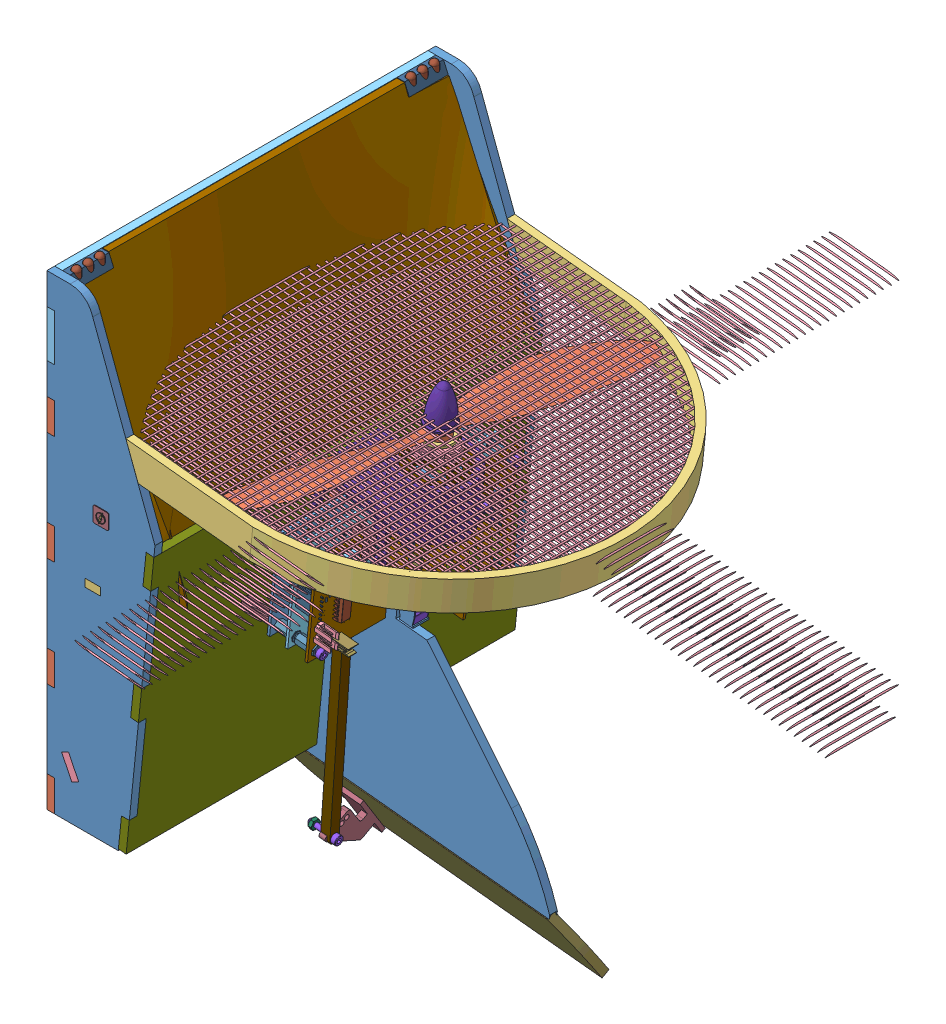
SolidWorks assembly AssTotaleSimu2, configuration Défaut. Lengths in mm. (continued)
Components (placement in the parent): (continued)
- AssStructSimu-1: AssStructSimu [Défaut] at (-125.7658 -1.8483 624.6548) x (1 0 0) z (0 0 -1) size (253.25 324.59 251.6) (continued)
  - AssCarte-1: AssCarte [Défaut] at (38.0121 147.1029 290.772) x (-0.101852 0.9948 0) z (0.9948 0.101852 0) size (66.52 130.57 98.72) (continued)
    - carte_onduleur_v3-1: carte_onduleur_v3 [Défaut] at (-131.8199 12.0892 20.7912) size (66.52 130.57 82.34) (continued)
      - RC2_2-1: RC2_2 [Défaut] at (-22 0.18 -0.803) x (-1 0 0) z (0 0 -1) size (2.34 1.04 0.5) (continued)
        - Open CASCADE STEP translator 6.8 1.12.1-1: Open CASCADE STEP translator 6.8 1.12.1 [Défaut] at origin size (2.34 1.04 0.5) (continued)
          - Pin_2_2-1: Pin_2_2 [Défaut] at origin size (0.51 1.02 0.5)
      - RC3_1-1: RC3_1 [Défaut] at (-20.9336 -14.5 -0.803) x (1 0 0) z (0 0 -1) size (2.34 1.04 0.5)
        - Open CASCADE STEP translator 6.8 1.12.1-1: Open CASCADE STEP translator 6.8 1.12.1 [Défaut] at origin size (2.34 1.04 0.5)
          - Body_1_3-1: Body_1_3 [Défaut] at origin size (2.29 1.04 0.43)
          - Pin_1_2-1: Pin_1_2 [Défaut] at (0.3048 0 0) x (-1 0 0) z (0 0 1) size (0.51 1.02 0.5)
          - Pin_2_2-1: Pin_2_2 [Défaut] at origin size (0.51 1.02 0.5)
      - RC3_2-1: RC3_2 [Défaut] at (-22.3 -14.5 -0.803) x (-1 0 0) z (0 0 -1) size (2.34 1.04 0.5)
        - Open CASCADE STEP translator 6.8 1.12.1-1: Open CASCADE STEP translator 6.8 1.12.1 [Défaut] at origin size (2.34 1.04 0.5)
          - Body_1_3-1: Body_1_3 [Défaut] at origin size (2.29 1.04 0.43)
          - Pin_1_2-1: Pin_1_2 [Défaut] at (0.3048 0 0) x (-1 0 0) z (0 0 1) size (0.51 1.02 0.5)
          - Pin_2_2-1: Pin_2_2 [Défaut] at origin size (0.51 1.02 0.5)
      - U_MES_CUR-1: U_MES_CUR [Défaut] at (-11.5 6.7816 0.803) size (2.54 2.41 0.76)
        - Open CASCADE STEP translator 6.8 1.32.1-1: Open CASCADE STEP translator 6.8 1.32.1 [Défaut] at origin size (2.54 2.41 0.76)
          - Body_1_5-1: Body_1_5 [Défaut] at origin size (2.54 1.27 0.71)
          - Pin_1_3-1: Pin_1_3 [Défaut] at (-2.1082 0.2286 0) x (0 -1 0) z (0 0 1) size (1.14 0.25 0.47)
          - Pin_2_3-1: Pin_2_3 [Défaut] at (-0.2032 2.1336 0) x (0 -1 0) z (0 0 1) size (1.14 0.25 0.47)
      - CARTE_ALIM-1: CARTE_ALIM [Défaut] at (-6.4 -57.2 0.803) size (60 130 18.35)
        - Open CASCADE STEP translator 6.8 1.33.1-1: Open CASCADE STEP translator 6.8 1.33.1 [Défaut] at origin size (60 130 18.35)
          - Body_1_6-1: Body_1_6 [Défaut] at (7 56 -12) size (60 130 18.35)
            - 1_3-1: 1_3 [Défaut] at origin size (60 130 1.61)
            - 13_3-1: 13_3 [Défaut] at (0.4717 -40.93 0.803) x (0 1 0) z (0 0 1) size (5.65 4.9 1.7)
              - =_[0_1_1_4]_3-1: =_[0_1_1_4]_3 [Défaut] at origin size (5.65 4.9 1.7)
                - 2-1: 2 [Défaut] at origin size (3.75 4.9 1.53)
                - 3-1: 3 [Défaut] at origin size (0.95 0.51 1.06)
                - 4-1: 4 [Défaut] at origin size (0.95 0.51 1.06)
                - 5_2-1: 5_2 [Défaut] at origin size (0.95 0.51 1.06)
                - 6-1: 6 [Défaut] at origin size (0.95 0.51 1.06)
                - 7-1: 7 [Défaut] at (10.8 -5.08 0) x (-1 0 0) z (0 0 1) size (0.95 0.51 1.06)
                - 8_2-1: 8_2 [Défaut] at (10.8 -2.54 0) x (-1 0 0) z (0 0 1) size (0.95 0.51 1.06)
                - 9-1: 9 [Défaut] at (10.8 0 0) x (-1 0 0) z (0 0 1) size (0.95 0.51 1.06)
                - 10-1: 10 [Défaut] at (10.8 2.54 0) x (-1 0 0) z (0 0 1) size (0.95 0.51 1.06)
                - 11_2-1: 11_2 [Défaut] at (5.4 -1.27 0) x (-1 0 0) z (0 0 1) size (4.25 2.34 1.06)
            - 18-1: 18 [Défaut] at (-2.5283 -37.23 0.803) x (0 -1 0) z (0 0 1) size (2.34 1.04 0.5)
              - =_[0_1_1_16]-1: =_[0_1_1_16] [Défaut] at origin size (2.34 1.04 0.5)
                - 14_2-1: 14_2 [Défaut] at origin size (2.29 1.04 0.43)
                - 15_2-1: 15_2 [Défaut] at (0.3048 0 0) x (-1 0 0) z (0 0 1) size (0.51 1.02 0.5)
                - 16_2-1: 16_2 [Défaut] at origin size (0.51 1.02 0.5)
            - 21_2-1: 21_2 [Défaut] at (-2.2263 -24.628 -0.803) x (1 0 0) z (0 0 -1) size (8.01 8 14.24)
              - =_[0_1_1_21]-1: =_[0_1_1_21] [Défaut] at origin size (8.01 8 14.24)
                - 19-1: 19 [Défaut] at (1.8 0 0) x (1 0 0) z (0 -1 0) size (8.01 14.24 8)
            - 23_2-1: 23_2 [Défaut] at (1.2381 -31.53 0.803) size (2.34 1.04 0.5)
              - =_[0_1_1_16]-1: =_[0_1_1_16] [Défaut] at origin size (2.34 1.04 0.5)
                - 14_2-1: 14_2 [Défaut] at origin size (2.29 1.04 0.43)
                - 15_2-1: 15_2 [Défaut] at (0.3048 0 0) x (-1 0 0) z (0 0 1) size (0.51 1.02 0.5)
                - 16_2-1: 16_2 [Défaut] at origin size (0.51 1.02 0.5)
            - 28-1: 28 [Défaut] at (5 29.8636 0.803) x (0 -1 0) z (0 0 1) size (3.35 1.3 0.55)
              - =_[0_1_1_25]_2-1: =_[0_1_1_25]_2 [Défaut] at origin size (3.35 1.3 0.55)
                - 24-1: 24 [Défaut] at origin size (3.3 1.3 0.48)
                - 25_2-1: 25_2 [Défaut] at (0.5588 0 0) x (-1 0 0) z (0 0 1) size (0.76 1.27 0.55)
                - 26_2-1: 26_2 [Défaut] at origin size (0.76 1.27 0.55)
            - 30-1: 30 [Défaut] at (6.7 29.8636 0.803) x (0 -1 0) z (0 0 1) size (2.34 1.04 0.5)
              - =_[0_1_1_16]-1: =_[0_1_1_16] [Défaut] at origin size (2.34 1.04 0.5)
                - 14_2-1: 14_2 [Défaut] at origin size (2.29 1.04 0.43)
                - 15_2-1: 15_2 [Défaut] at (0.3048 0 0) x (-1 0 0) z (0 0 1) size (0.51 1.02 0.5)
                - 16_2-1: 16_2 [Défaut] at origin size (0.51 1.02 0.5)
            - 35_2-1: 35_2 [Défaut] at (-2.5 -46.37 0.803) x (0 1 0) z (0 0 1) size (3.4 2.06 0.79)
              - =_[0_1_1_31]-1: =_[0_1_1_31] [Défaut] at origin size (3.4 2.06 0.79)
                - 31_2-1: 31_2 [Défaut] at origin size (3.3 2.06 0.69)
                - 32_3-1: 32_3 [Défaut] at (0.5588 0 0) x (-1 0 0) z (0 0 1) size (0.81 2.03 0.79)
                - 33_3-1: 33_3 [Défaut] at origin size (0.81 2.03 0.79)
            - 37-1: 37 [Défaut] at (5 31.43 0.803) x (0 1 0) z (0 0 1) size (2.34 1.04 0.5)
              - =_[0_1_1_16]-1: =_[0_1_1_16] [Défaut] at origin size (2.34 1.04 0.5)
                - 14_2-1: 14_2 [Défaut] at origin size (2.29 1.04 0.43)
                - 15_2-1: 15_2 [Défaut] at (0.3048 0 0) x (-1 0 0) z (0 0 1) size (0.51 1.02 0.5)
                - 16_2-1: 16_2 [Défaut] at origin size (0.51 1.02 0.5)
            - 39-1: 39 [Défaut] at (-0.2 35.63 0.803) x (-1 0 0) z (0 0 1) size (2.34 1.04 0.5)
              - =_[0_1_1_16]-1: =_[0_1_1_16] [Défaut] at origin size (2.34 1.04 0.5)
                - 14_2-1: 14_2 [Défaut] at origin size (2.29 1.04 0.43)
                - 15_2-1: 15_2 [Défaut] at (0.3048 0 0) x (-1 0 0) z (0 0 1) size (0.51 1.02 0.5)
                - 16_2-1: 16_2 [Défaut] at origin size (0.51 1.02 0.5)
            - 41-1: 41 [Défaut] at (2.9 -45.5036 0.803) x (0 1 0) z (0 0 1) size (2.34 1.04 0.5)
              - =_[0_1_1_16]-1: =_[0_1_1_16] [Défaut] at origin size (2.34 1.04 0.5)
                - 14_2-1: 14_2 [Défaut] at origin size (2.29 1.04 0.43)
                - 15_2-1: 15_2 [Défaut] at (0.3048 0 0) x (-1 0 0) z (0 0 1) size (0.51 1.02 0.5)
                - 16_2-1: 16_2 [Défaut] at origin size (0.51 1.02 0.5)
            - 43-1: 43 [Défaut] at (17.1348 -42.6272 0.803) x (0 1 0) z (0 0 1) size (2.34 1.04 0.5)
              - =_[0_1_1_16]-1: =_[0_1_1_16] [Défaut] at origin size (2.34 1.04 0.5)
                - 14_2-1: 14_2 [Défaut] at origin size (2.29 1.04 0.43)
                - 15_2-1: 15_2 [Défaut] at (0.3048 0 0) x (-1 0 0) z (0 0 1) size (0.51 1.02 0.5)
                - 16_2-1: 16_2 [Défaut] at origin size (0.51 1.02 0.5)
            - 48_2-1: 48_2 [Défaut] at (-5.4717 -39.01 0.803) x (-1 0 0) z (0 0 1) size (4.19 3.4 1.75)
              - =_[0_1_1_40]-1: =_[0_1_1_40] [Défaut] at origin size (4.19 3.4 1.75)
                - 44_2-1: 44_2 [Défaut] at origin size (3.75 3.38 1.73)
                - 45_2-1: 45_2 [Défaut] at (0.438 0 0) x (-1 0 0) z (0 0 1) size (0.53 3.4 1.75)
                - 46_2-1: 46_2 [Défaut] at origin size (0.52 3.4 1.75)
            - 53-1: 53 [Défaut] at (0.9 35.63 0.803) size (2.34 1.04 0.5)
              - =_[0_1_1_45]-1: =_[0_1_1_45] [Défaut] at origin size (2.34 1.04 0.5)
                - 49_3-1: 49_3 [Défaut] at origin size (2.29 1.04 0.43)
                - 50-1: 50 [Défaut] at (0.3048 0 0) x (-1 0 0) z (0 0 1) size (0.51 1.02 0.5)
                - 51-1: 51 [Défaut] at origin size (0.51 1.02 0.5)
            - 55_2-1: 55_2 [Défaut] at (1.3 -45.5036 0.803) x (0 1 0) z (0 0 1) size (2.34 1.04 0.5)
              - =_[0_1_1_45]-1: =_[0_1_1_45] [Défaut] at origin size (2.34 1.04 0.5)
                - 49_3-1: 49_3 [Défaut] at origin size (2.29 1.04 0.43)
                - 50-1: 50 [Défaut] at (0.3048 0 0) x (-1 0 0) z (0 0 1) size (0.51 1.02 0.5)
                - 51-1: 51 [Défaut] at origin size (0.51 1.02 0.5)
            - 57_3-1: 57_3 [Défaut] at (17.2348 -43.9936 0.803) x (0 -1 0) z (0 0 1) size (2.34 1.04 0.5)
              - =_[0_1_1_45]-1: =_[0_1_1_45] [Défaut] at origin size (2.34 1.04 0.5)
                - 49_3-1: 49_3 [Défaut] at origin size (2.29 1.04 0.43)
                - 50-1: 50 [Défaut] at (0.3048 0 0) x (-1 0 0) z (0 0 1) size (0.51 1.02 0.5)
                - 51-1: 51 [Défaut] at origin size (0.51 1.02 0.5)
            - 65-1: 65 [Défaut] at (-4.8 30.93 0.803) x (-1 0 0) z (0 0 1) size (14.64 9.83 4.25)
              - =_[0_1_1_52]-1: =_[0_1_1_52] [Défaut] at origin size (14.64 9.83 4.25)
                - 63_2-1: 63_2 [Défaut] at (3 0 0) x (0 -1 0) z (0 0 1) size (9.83 14.64 4.25)
                  - =_[0_1_1_3]_5-1: =_[0_1_1_3]_5 [Défaut] at origin size (9.83 9.05 4.21)
                  - =_[0_1_1_4]_5-1: =_[0_1_1_4]_5 [Défaut] at origin size (9.48 7.76 1.21)
                  - =_[0_1_1_5]_5-1: =_[0_1_1_5]_5 [Défaut] at origin size (1.36 6.01 3.08)
                  - =_[0_1_1_6]_3-1: =_[0_1_1_6]_3 [Défaut] at origin size (1.36 6.01 3.08)
                  - =_[0_1_1_7]_3-1: =_[0_1_1_7]_3 [Défaut] at origin size (1.06 6.01 3.08)
            - 67-1: 67 [Défaut] at (13.5933 -37.5272 0.803) x (-1 0 0) z (0 0 1) size (2.34 1.04 0.5)
              - =_[0_1_1_16]-1: =_[0_1_1_16] [Défaut] at origin size (2.34 1.04 0.5)
                - 14_2-1: 14_2 [Défaut] at origin size (2.29 1.04 0.43)
                - 15_2-1: 15_2 [Défaut] at (0.3048 0 0) x (-1 0 0) z (0 0 1) size (0.51 1.02 0.5)
                - 16_2-1: 16_2 [Défaut] at origin size (0.51 1.02 0.5)
            - 70_2-1: 70_2 [Défaut] at (18.2733 -29.7272 0.803) x (0 1 0) z (0 0 1) size (6.06 4.95 1.88)
              - =_[0_1_1_61]-1: =_[0_1_1_61] [Défaut] at origin size (6.06 4.95 1.88)
                - 68-1: 68 [Défaut] x (1 0 0) z (0 -1 0) size (6.06 1.88 4.95)
            - 83-1: 83 [Défaut] at (-21.2 -38.07 0.803) x (-1 0 0) z (0 0 1) size (2.7 5.2 1.11)
              - =_[0_1_1_64]-1: =_[0_1_1_64] [Défaut] at origin size (2.7 5.2 1.11)
                - 84_2-1: 84_2 [Défaut] at (1.2 -4 0) x (0 1 0) z (0 0 1) size (5.2 2.7 1.11)
                  - =_[0_1_1_3]_6-1: =_[0_1_1_3]_6 [Défaut] at origin size (0.39 0.64 0.01)
                  - =_[0_1_1_4]_6-1: =_[0_1_1_4]_6 [Défaut] at origin size (0.6 1.9 0.2)
                  - =_[0_1_1_5]_6-1: =_[0_1_1_5]_6 [Défaut] at origin size (0.21 0.08 0.01)
                  - =_[0_1_1_6]_4-1: =_[0_1_1_6]_4 [Défaut] at origin size (0.6 1.9 0.2)
                  - =_[0_1_1_7]_4-1: =_[0_1_1_7]_4 [Défaut] at origin size (0.46 0.68 0.01)
                  - =_[0_1_1_8]_3-1: =_[0_1_1_8]_3 [Défaut] at origin size (0.38 0.66 0.01)
                  - =_[0_1_1_9]_2-1: =_[0_1_1_9]_2 [Défaut] at origin size (0.2 0.62 0.01)
                  - =_[0_1_1_10]_2-1: =_[0_1_1_10]_2 [Défaut] at origin size (4 2.7 1.1)
                  - =_[0_1_1_11]_2-1: =_[0_1_1_11]_2 [Défaut] at origin size (0.46 0.63 0.01)
                  - =_[0_1_1_12]_2-1: =_[0_1_1_12]_2 [Défaut] at origin size (0.56 0.68 0.01)
            - 86_2-1: 86_2 [Défaut] at (12.8933 -35.4272 0.803) x (0 1 0) z (0 0 1) size (2.7 5.2 1.11)
              - =_[0_1_1_77]-1: =_[0_1_1_77] [Défaut] at origin size (2.7 5.2 1.11)
                - 84_2-1: 84_2 [Défaut] at (1.2 -4 0) x (0 1 0) z (0 0 1) size (5.2 2.7 1.11)
                  - =_[0_1_1_3]_6-1: =_[0_1_1_3]_6 [Défaut] at origin size (0.39 0.64 0.01)
                  - =_[0_1_1_4]_6-1: =_[0_1_1_4]_6 [Défaut] at origin size (0.6 1.9 0.2)
                  - =_[0_1_1_5]_6-1: =_[0_1_1_5]_6 [Défaut] at origin size (0.21 0.08 0.01)
                  - =_[0_1_1_6]_4-1: =_[0_1_1_6]_4 [Défaut] at origin size (0.6 1.9 0.2)
                  - =_[0_1_1_7]_4-1: =_[0_1_1_7]_4 [Défaut] at origin size (0.46 0.68 0.01)
                  - =_[0_1_1_8]_3-1: =_[0_1_1_8]_3 [Défaut] at origin size (0.38 0.66 0.01)
                  - =_[0_1_1_9]_2-1: =_[0_1_1_9]_2 [Défaut] at origin size (0.2 0.62 0.01)
                  - =_[0_1_1_10]_2-1: =_[0_1_1_10]_2 [Défaut] at origin size (4 2.7 1.1)
                  - =_[0_1_1_11]_2-1: =_[0_1_1_11]_2 [Défaut] at origin size (0.46 0.63 0.01)
                  - =_[0_1_1_12]_2-1: =_[0_1_1_12]_2 [Défaut] at origin size (0.56 0.68 0.01)
            - 92_2-1: 92_2 [Défaut] at (20.9933 -39.3272 0.803) x (0 -1 0) z (0 0 1) size (2.79 1.98 0.64)
              - =_[0_1_1_79]-1: =_[0_1_1_79] [Défaut] at origin size (2.79 1.98 0.64)
                - 87-1: 87 [Défaut] at origin size (2.79 1.02 0.58)
                - 88-1: 88 [Défaut] x (0 -1 0) z (0 0 1) size (0.42 0.38 0.38)
                - 89-1: 89 [Défaut] at (-2.8448 -0.9652 0) x (0 1 0) z (0 0 1) size (0.55 0.38 0.38)
                - 90-1: 90 [Défaut] at (-0.9652 -2.8448 0) x (0 1 0) z (0 0 1) size (0.55 0.38 0.38)
            - 98-1: 98 [Défaut] at (-17.7 -48.47 0.803) x (0 -1 0) z (0 0 1) size (2.54 1.98 0.64)
              - =_[0_1_1_85]-1: =_[0_1_1_85] [Défaut] at origin size (2.54 1.98 0.64)
                - 93-1: 93 [Défaut] at origin size (2.54 1.14 0.58)
                - 94-1: 94 [Défaut] x (0 -1 0) z (0 0 1) size (0.43 0.51 0.38)
                - 95-1: 95 [Défaut] at (1.8796 1.8796 0) x (0 -1 0) z (0 0 1) size (0.43 0.51 0.38)
                - 96-1: 96 [Défaut] at (-0.9652 -2.8448 0) x (0 1 0) z (0 0 1) size (0.41 0.51 0.38)
            - 100-1: 100 [Défaut] at (24.3933 -43.2272 0.803) size (2.79 1.98 0.64)
              - =_[0_1_1_79]-1: =_[0_1_1_79] [Défaut] at origin size (2.79 1.98 0.64)
                - 87-1: 87 [Défaut] at origin size (2.79 1.02 0.58)
                - 88-1: 88 [Défaut] x (0 -1 0) z (0 0 1) size (0.42 0.38 0.38)
                - 89-1: 89 [Défaut] at (-2.8448 -0.9652 0) x (0 1 0) z (0 0 1) size (0.55 0.38 0.38)
                - 90-1: 90 [Défaut] at (-0.9652 -2.8448 0) x (0 1 0) z (0 0 1) size (0.55 0.38 0.38)
            - 102-1: 102 [Défaut] at (21.4933 -44.4272 0.803) x (0 -1 0) z (0 0 1) size (2.79 1.98 0.64)
              - =_[0_1_1_79]-1: =_[0_1_1_79] [Défaut] at origin size (2.79 1.98 0.64)
                - 87-1: 87 [Défaut] at origin size (2.79 1.02 0.58)
                - 88-1: 88 [Défaut] x (0 -1 0) z (0 0 1) size (0.42 0.38 0.38)
                - 89-1: 89 [Défaut] at (-2.8448 -0.9652 0) x (0 1 0) z (0 0 1) size (0.55 0.38 0.38)
                - 90-1: 90 [Défaut] at (-0.9652 -2.8448 0) x (0 1 0) z (0 0 1) size (0.55 0.38 0.38)
            - 107-1: 107 [Défaut] at (23.1933 -29.1272 -0.803) x (0 1 0) z (0 0 -1) size (9.6 14.35 5)
              - =_[0_1_1_93]-1: =_[0_1_1_93] [Défaut] at origin size (9.6 14.35 5)
                - 105-1: 105 [Défaut] at (0.5 -1 2) x (-1 0 0) z (0 0 1) size (9.6 14.35 5)
                  - =_[0_1_1_3]_7-1: =_[0_1_1_3]_7 [Défaut] at origin size (9.6 12.75 5)
                  - =_[0_1_1_4]_7-1: =_[0_1_1_4]_7 [Défaut] at origin size (2.2 1.6 2.2)
            - 109-1: 109 [Défaut] at (25.4933 -41.1272 0.803) x (-1 0 0) z (0 0 1) size (2.34 1.04 0.5)
              - =_[0_1_1_45]-1: =_[0_1_1_45] [Défaut] at origin size (2.34 1.04 0.5)
                - 49_3-1: 49_3 [Défaut] at origin size (2.29 1.04 0.43)
                - 50-1: 50 [Défaut] at (0.3048 0 0) x (-1 0 0) z (0 0 1) size (0.51 1.02 0.5)
                - 51-1: 51 [Défaut] at origin size (0.51 1.02 0.5)
            - 111-1: 111 [Défaut] at (22.0269 -41.8272 0.803) x (-1 0 0) z (0 0 1) size (2.34 1.04 0.5)
              - =_[0_1_1_45]-1: =_[0_1_1_45] [Défaut] at origin size (2.34 1.04 0.5)
                - 49_3-1: 49_3 [Défaut] at origin size (2.29 1.04 0.43)
                - 50-1: 50 [Défaut] at (0.3048 0 0) x (-1 0 0) z (0 0 1) size (0.51 1.02 0.5)
                - 51-1: 51 [Défaut] at origin size (0.51 1.02 0.5)
            - 113-1: 113 [Défaut] at (-24.8 -36.7036 0.803) x (0 1 0) z (0 0 1) size (2.34 1.04 0.5)
              - =_[0_1_1_45]-1: =_[0_1_1_45] [Défaut] at origin size (2.34 1.04 0.5)
                - 49_3-1: 49_3 [Défaut] at origin size (2.29 1.04 0.43)
                - 50-1: 50 [Défaut] at (0.3048 0 0) x (-1 0 0) z (0 0 1) size (0.51 1.02 0.5)
                - 51-1: 51 [Défaut] at origin size (0.51 1.02 0.5)
            - 115-1: 115 [Défaut] at (-24.8 -40.3036 0.803) x (0 1 0) z (0 0 1) size (2.34 1.04 0.5)
              - =_[0_1_1_45]-1: =_[0_1_1_45] [Défaut] at origin size (2.34 1.04 0.5)
                - 49_3-1: 49_3 [Défaut] at origin size (2.29 1.04 0.43)
                - 50-1: 50 [Défaut] at (0.3048 0 0) x (-1 0 0) z (0 0 1) size (0.51 1.02 0.5)
                - 51-1: 51 [Défaut] at origin size (0.51 1.02 0.5)
            - 117-1: 117 [Défaut] at (-16 -48.27 0.803) x (0 -1 0) z (0 0 1) size (2.34 1.04 0.5)
              - =_[0_1_1_45]-1: =_[0_1_1_45] [Défaut] at origin size (2.34 1.04 0.5)
                - 49_3-1: 49_3 [Défaut] at origin size (2.29 1.04 0.43)
                - 50-1: 50 [Défaut] at (0.3048 0 0) x (-1 0 0) z (0 0 1) size (0.51 1.02 0.5)
                - 51-1: 51 [Défaut] at origin size (0.51 1.02 0.5)
            - 119-1: 119 [Défaut] at (-22.5189 -47.87 0.803) x (-1 0 0) z (0 0 1) size (2.34 1.04 0.5)
              - =_[0_1_1_45]-1: =_[0_1_1_45] [Défaut] at origin size (2.34 1.04 0.5)
                - 49_3-1: 49_3 [Défaut] at origin size (2.29 1.04 0.43)
                - 50-1: 50 [Défaut] at (0.3048 0 0) x (-1 0 0) z (0 0 1) size (0.51 1.02 0.5)
                - 51-1: 51 [Défaut] at origin size (0.51 1.02 0.5)
            - 121-1: 121 [Défaut] at (22.3933 -38.9272 0.803) size (2.34 1.04 0.5)
              - =_[0_1_1_45]-1: =_[0_1_1_45] [Défaut] at origin size (2.34 1.04 0.5)
                - 49_3-1: 49_3 [Défaut] at origin size (2.29 1.04 0.43)
                - 50-1: 50 [Défaut] at (0.3048 0 0) x (-1 0 0) z (0 0 1) size (0.51 1.02 0.5)
                - 51-1: 51 [Défaut] at origin size (0.51 1.02 0.5)
            - 123-1: 123 [Défaut] at (22.0933 -36.4272 0.803) x (-1 0 0) z (0 0 1) size (2.34 1.04 0.5)
              - =_[0_1_1_45]-1: =_[0_1_1_45] [Défaut] at origin size (2.34 1.04 0.5)
                - 49_3-1: 49_3 [Défaut] at origin size (2.29 1.04 0.43)
                - 50-1: 50 [Défaut] at (0.3048 0 0) x (-1 0 0) z (0 0 1) size (0.51 1.02 0.5)
                - 51-1: 51 [Défaut] at origin size (0.51 1.02 0.5)
            - 125-1: 125 [Défaut] at (22.3933 -32.0272 0.803) x (0 -1 0) z (0 0 1) size (2.34 1.04 0.5)
              - =_[0_1_1_45]-1: =_[0_1_1_45] [Défaut] at origin size (2.34 1.04 0.5)
                - 49_3-1: 49_3 [Défaut] at origin size (2.29 1.04 0.43)
                - 50-1: 50 [Défaut] at (0.3048 0 0) x (-1 0 0) z (0 0 1) size (0.51 1.02 0.5)
                - 51-1: 51 [Défaut] at origin size (0.51 1.02 0.5)
            - 127-1: 127 [Défaut] at (17.9597 -23.1272 0.803) size (2.34 1.04 0.5)
              - =_[0_1_1_16]-1: =_[0_1_1_16] [Défaut] at origin size (2.34 1.04 0.5)
                - 14_2-1: 14_2 [Défaut] at origin size (2.29 1.04 0.43)
                - 15_2-1: 15_2 [Défaut] at (0.3048 0 0) x (-1 0 0) z (0 0 1) size (0.51 1.02 0.5)
                - 16_2-1: 16_2 [Défaut] at origin size (0.51 1.02 0.5)
            - 129-1: 129 [Défaut] at (20.0269 -24.9272 0.803) x (-1 0 0) z (0 0 1) size (2.34 1.04 0.5)
              - =_[0_1_1_16]-1: =_[0_1_1_16] [Défaut] at origin size (2.34 1.04 0.5)
                - 14_2-1: 14_2 [Défaut] at origin size (2.29 1.04 0.43)
                - 15_2-1: 15_2 [Défaut] at (0.3048 0 0) x (-1 0 0) z (0 0 1) size (0.51 1.02 0.5)
                - 16_2-1: 16_2 [Défaut] at origin size (0.51 1.02 0.5)
            - 131-1: 131 [Défaut] at (16.9933 -37.5272 0.803) x (-1 0 0) z (0 0 1) size (2.34 1.04 0.5)
              - =_[0_1_1_45]-1: =_[0_1_1_45] [Défaut] at origin size (2.34 1.04 0.5)
                - 49_3-1: 49_3 [Défaut] at origin size (2.29 1.04 0.43)
                - 50-1: 50 [Défaut] at (0.3048 0 0) x (-1 0 0) z (0 0 1) size (0.51 1.02 0.5)
                - 51-1: 51 [Défaut] at origin size (0.51 1.02 0.5)
            - 136-1: 136 [Défaut] at (3.2957 -29.23 0.803) x (-1 0 0) z (0 0 1) size (4.78 2.79 2.03)
              - =_[0_1_1_110]_2-1: =_[0_1_1_110]_2 [Défaut] at origin size (4.78 2.79 2.03)
                - 132-1: 132 [Défaut] at origin size (4.32 2.79 1.78)
                - 133-1: 133 [Défaut] at (0.4572 0 0) x (-1 0 0) z (0 0 1) size (1.02 1.27 1.32)
                - 134-1: 134 [Défaut] at origin size (1.02 1.27 1.32)
            - 141-1: 141 [Défaut] at (0.2436 -33.3673 0.803) size (3.35 1.3 0.55)
              - =_[0_1_1_115]_2-1: =_[0_1_1_115]_2 [Défaut] at origin size (3.35 1.3 0.55)
                - 137-1: 137 [Défaut] at origin size (3.3 1.3 0.48)
                - 138-1: 138 [Défaut] at (0.5588 0 0) x (-1 0 0) z (0 0 1) size (0.76 1.27 0.55)
                - 139-1: 139 [Défaut] at origin size (0.76 1.27 0.55)
            - 143_2-1: 143_2 [Défaut] at (-0.3 -45.47 0.803) x (0 1 0) z (0 0 1) size (2.34 1.04 0.5)
              - =_[0_1_1_16]-1: =_[0_1_1_16] [Défaut] at origin size (2.34 1.04 0.5)
                - 14_2-1: 14_2 [Défaut] at origin size (2.29 1.04 0.43)
                - 15_2-1: 15_2 [Défaut] at (0.3048 0 0) x (-1 0 0) z (0 0 1) size (0.51 1.02 0.5)
                - 16_2-1: 16_2 [Défaut] at origin size (0.51 1.02 0.5)
            - 145-1: 145 [Défaut] at (6.6 31.13 0.803) x (0 1 0) z (0 0 1) size (3.35 1.3 0.55)
              - =_[0_1_1_25]_2-1: =_[0_1_1_25]_2 [Défaut] at origin size (3.35 1.3 0.55)
                - 24-1: 24 [Défaut] at origin size (3.3 1.3 0.48)
                - 25_2-1: 25_2 [Défaut] at (0.5588 0 0) x (-1 0 0) z (0 0 1) size (0.76 1.27 0.55)
                - 26_2-1: 26_2 [Défaut] at origin size (0.76 1.27 0.55)
            - 148-1: 148 [Défaut] at (-7.5 -56.57 0.803) size (15.24 2.54 7.37)
              - =_[0_1_1_122]_2-1: =_[0_1_1_122]_2 [Défaut] at origin size (15.24 2.54 7.37)
                - 146-1: 146 [Défaut] at (6.3 0 1) x (1 0 0) z (0 -1 0) size (15.24 7.37 2.54)
      - COMP1-1: COMP1 [Défaut] at (-16.3 -36.2 0.803) x (-1 0 0) z (0 0 1) size (2.03 1.88 0.51)
        - Open CASCADE STEP translator 6.8 1.34.1-1: Open CASCADE STEP translator 6.8 1.34.1 [Défaut] at origin size (2.03 1.88 0.51)
          - Body_1_6-1: Body_1_6 [Défaut] at origin size (2.03 1.02 0.46)
          - Pin_1_4-1: Pin_1_4 [Défaut] x (0 1 0) z (0 0 1) size (0.45 0.25 0.32)
          - Pin_2_4-1: Pin_2_4 [Défaut] at (0.65 -0.65 0) x (0 1 0) z (0 0 1) size (0.45 0.25 0.32)
          - Pin_3-1: Pin_3 [Défaut] at (1.3 -1.3 0) x (0 1 0) z (0 0 1) size (0.45 0.25 0.32)
          - Pin_4-1: Pin_4 [Défaut] at (-0.5 3.1 0) x (0 -1 0) z (0 0 1) size (0.41 0.25 0.32)
          - Pin_5-1: Pin_5 [Défaut] at (-1.8 1.8 0) x (0 -1 0) z (0 0 1) size (0.41 0.25 0.32)
      - COMP2-1: COMP2 [Défaut] at (-14.3 -9.6 0.803) x (-1 0 0) z (0 0 1) size (2.03 1.88 0.51)
        - Open CASCADE STEP translator 6.8 1.34.1-1: Open CASCADE STEP translator 6.8 1.34.1 [Défaut] at origin size (2.03 1.88 0.51)
          - Body_1_6-1: Body_1_6 [Défaut] at origin size (2.03 1.02 0.46)
          - Pin_1_4-1: Pin_1_4 [Défaut] x (0 1 0) z (0 0 1) size (0.45 0.25 0.32)
          - Pin_2_4-1: Pin_2_4 [Défaut] at (0.65 -0.65 0) x (0 1 0) z (0 0 1) size (0.45 0.25 0.32)
          - Pin_3-1: Pin_3 [Défaut] at (1.3 -1.3 0) x (0 1 0) z (0 0 1) size (0.45 0.25 0.32)
          - Pin_4-1: Pin_4 [Défaut] at (-0.5 3.1 0) x (0 -1 0) z (0 0 1) size (0.41 0.25 0.32)
          - Pin_5-1: Pin_5 [Défaut] at (-1.8 1.8 0) x (0 -1 0) z (0 0 1) size (0.41 0.25 0.32)
      - COMP3-1: COMP3 [Défaut] at (-15.9 -23.2 0.803) x (-1 0 0) z (0 0 1) size (2.03 1.88 0.51)
        - Open CASCADE STEP translator 6.8 1.34.1-1: Open CASCADE STEP translator 6.8 1.34.1 [Défaut] at origin size (2.03 1.88 0.51)
          - Body_1_6-1: Body_1_6 [Défaut] at origin size (2.03 1.02 0.46)
          - Pin_1_4-1: Pin_1_4 [Défaut] x (0 1 0) z (0 0 1) size (0.45 0.25 0.32)
          - Pin_2_4-1: Pin_2_4 [Défaut] at (0.65 -0.65 0) x (0 1 0) z (0 0 1) size (0.45 0.25 0.32)
          - Pin_3-1: Pin_3 [Défaut] at (1.3 -1.3 0) x (0 1 0) z (0 0 1) size (0.45 0.25 0.32)
          - Pin_4-1: Pin_4 [Défaut] at (-0.5 3.1 0) x (0 -1 0) z (0 0 1) size (0.41 0.25 0.32)
          - Pin_5-1: Pin_5 [Défaut] at (-1.8 1.8 0) x (0 -1 0) z (0 0 1) size (0.41 0.25 0.32)
      - CP1-1: CP1 [Défaut] at (-18.9 -38.2 0.803) x (0 1 0) z (0 0 1) size (2.34 1.04 0.5)
        - Open CASCADE STEP translator 6.8 1.6.1-1: Open CASCADE STEP translator 6.8 1.6.1 [Défaut] at origin size (2.34 1.04 0.5)
          - Body_1-1: Body_1 [Défaut] at origin size (2.29 1.04 0.43)
          - Pin_1-1: Pin_1 [Défaut] at (0.3048 0 0) x (-1 0 0) z (0 0 1) size (0.51 1.02 0.5)
          - Pin_2-1: Pin_2 [Défaut] at origin size (0.51 1.02 0.5)
      - CP2-1: CP2 [Défaut] at (-16.9 -11.6 0.803) x (0 1 0) z (0 0 1) size (2.34 1.04 0.5)
        - Open CASCADE STEP translator 6.8 1.6.1-1: Open CASCADE STEP translator 6.8 1.6.1 [Défaut] at origin size (2.34 1.04 0.5)
          - Body_1-1: Body_1 [Défaut] at origin size (2.29 1.04 0.43)
          - Pin_1-1: Pin_1 [Défaut] at (0.3048 0 0) x (-1 0 0) z (0 0 1) size (0.51 1.02 0.5)
          - Pin_2-1: Pin_2 [Défaut] at origin size (0.51 1.02 0.5)
      - CP3-1: CP3 [Défaut] at (-18.5 -25.2 0.803) x (0 1 0) z (0 0 1) size (2.34 1.04 0.5)
        - Open CASCADE STEP translator 6.8 1.6.1-1: Open CASCADE STEP translator 6.8 1.6.1 [Défaut] at origin size (2.34 1.04 0.5)
          - Body_1-1: Body_1 [Défaut] at origin size (2.29 1.04 0.43)
          - Pin_1-1: Pin_1 [Défaut] at (0.3048 0 0) x (-1 0 0) z (0 0 1) size (0.51 1.02 0.5)
          - Pin_2-1: Pin_2 [Défaut] at origin size (0.51 1.02 0.5)
      - C_DEC_COM1-1: C_DEC_COM1 [Défaut] at (-15 -36 0.803) x (0 -1 0) z (0 0 1) size (2.34 1.04 0.5)
        - Open CASCADE STEP translator 6.8 1.6.1-1: Open CASCADE STEP translator 6.8 1.6.1 [Défaut] at origin size (2.34 1.04 0.5)
          - Body_1-1: Body_1 [Défaut] at origin size (2.29 1.04 0.43)
          - Pin_1-1: Pin_1 [Défaut] at (0.3048 0 0) x (-1 0 0) z (0 0 1) size (0.51 1.02 0.5)
          - Pin_2-1: Pin_2 [Défaut] at origin size (0.51 1.02 0.5)
      - C_DEC_COMP2-1: C_DEC_COMP2 [Défaut] at (-13 -9.3 0.803) x (0 -1 0) z (0 0 1) size (2.34 1.04 0.5)
        - Open CASCADE STEP translator 6.8 1.6.1-1: Open CASCADE STEP translator 6.8 1.6.1 [Défaut] at origin size (2.34 1.04 0.5)
          - Body_1-1: Body_1 [Défaut] at origin size (2.29 1.04 0.43)
          - Pin_1-1: Pin_1 [Défaut] at (0.3048 0 0) x (-1 0 0) z (0 0 1) size (0.51 1.02 0.5)
          - Pin_2-1: Pin_2 [Défaut] at origin size (0.51 1.02 0.5)
      - C_DEC_COMP3-1: C_DEC_COMP3 [Défaut] at (-14.6 -22.9 0.803) x (0 -1 0) z (0 0 1) size (2.34 1.04 0.5)
        - Open CASCADE STEP translator 6.8 1.6.1-1: Open CASCADE STEP translator 6.8 1.6.1 [Défaut] at origin size (2.34 1.04 0.5)
          - Body_1-1: Body_1 [Défaut] at origin size (2.29 1.04 0.43)
          - Pin_1-1: Pin_1 [Défaut] at (0.3048 0 0) x (-1 0 0) z (0 0 1) size (0.51 1.02 0.5)
          - Pin_2-1: Pin_2 [Défaut] at origin size (0.51 1.02 0.5)
      - D_VBAT-1: D_VBAT [Défaut] at (-1.2 46.4 0.803) x (0 -1 0) z (0 0 1) size (2.34 1.04 0.5)
        - Open CASCADE STEP translator 6.8 1.6.1-1: Open CASCADE STEP translator 6.8 1.6.1 [Défaut] at origin size (2.34 1.04 0.5)
          - Body_1-1: Body_1 [Défaut] at origin size (2.29 1.04 0.43)
          - Pin_1-1: Pin_1 [Défaut] at (0.3048 0 0) x (-1 0 0) z (0 0 1) size (0.51 1.02 0.5)
          - Pin_2-1: Pin_2 [Défaut] at origin size (0.51 1.02 0.5)
      - D_3V-1: D_3V [Défaut] at (1.3 46.3 0.803) x (0 -1 0) z (0 0 1) size (2.34 1.04 0.5)
        - Open CASCADE STEP translator 6.8 1.6.1-1: Open CASCADE STEP translator 6.8 1.6.1 [Défaut] at origin size (2.34 1.04 0.5)
          - Body_1-1: Body_1 [Défaut] at origin size (2.29 1.04 0.43)
          - Pin_1-1: Pin_1 [Défaut] at (0.3048 0 0) x (-1 0 0) z (0 0 1) size (0.51 1.02 0.5)
          - Pin_2-1: Pin_2 [Défaut] at origin size (0.51 1.02 0.5)
      - D_5V-1: D_5V [Défaut] at (-3.7 46.4 0.803) x (0 -1 0) z (0 0 1) size (2.34 1.04 0.5)
        - Open CASCADE STEP translator 6.8 1.6.1-1: Open CASCADE STEP translator 6.8 1.6.1 [Défaut] at origin size (2.34 1.04 0.5)
          - Body_1-1: Body_1 [Défaut] at origin size (2.29 1.04 0.43)
          - Pin_1-1: Pin_1 [Défaut] at (0.3048 0 0) x (-1 0 0) z (0 0 1) size (0.51 1.02 0.5)
          - Pin_2-1: Pin_2 [Défaut] at origin size (0.51 1.02 0.5)
      - R1_1-1: R1_1 [Défaut] at (-20.2 -36.1 0.803) x (-1 0 0) z (0 0 1) size (2.34 1.04 0.5)
        - Open CASCADE STEP translator 6.8 1.12.1-1: Open CASCADE STEP translator 6.8 1.12.1 [Défaut] at origin size (2.34 1.04 0.5)
          - Body_1_3-1: Body_1_3 [Défaut] at origin size (2.29 1.04 0.43)
          - Pin_1_2-1: Pin_1_2 [Défaut] at (0.3048 0 0) x (-1 0 0) z (0 0 1) size (0.51 1.02 0.5)
          - Pin_2_2-1: Pin_2_2 [Défaut] at origin size (0.51 1.02 0.5)
      - R1_2-1: R1_2 [Défaut] at (-15.5 -34.6 0.803) x (-1 0 0) z (0 0 1) size (2.34 1.04 0.5)
        - Open CASCADE STEP translator 6.8 1.12.1-1: Open CASCADE STEP translator 6.8 1.12.1 [Défaut] at origin size (2.34 1.04 0.5)
          - Body_1_3-1: Body_1_3 [Défaut] at origin size (2.29 1.04 0.43)
          - Pin_1_2-1: Pin_1_2 [Défaut] at (0.3048 0 0) x (-1 0 0) z (0 0 1) size (0.51 1.02 0.5)
          - Pin_2_2-1: Pin_2_2 [Défaut] at origin size (0.51 1.02 0.5)
      - R1_3-1: R1_3 [Défaut] at (-20.3 -39.9 0.803) x (-1 0 0) z (0 0 1) size (2.34 1.04 0.5)
        - Open CASCADE STEP translator 6.8 1.12.1-1: Open CASCADE STEP translator 6.8 1.12.1 [Défaut] at origin size (2.34 1.04 0.5)
          - Body_1_3-1: Body_1_3 [Défaut] at origin size (2.29 1.04 0.43)
          - Pin_1_2-1: Pin_1_2 [Défaut] at (0.3048 0 0) x (-1 0 0) z (0 0 1) size (0.51 1.02 0.5)
          - Pin_2_2-1: Pin_2_2 [Défaut] at origin size (0.51 1.02 0.5)
      - R1_4-1: R1_4 [Défaut] at (-20.3 -38.1 0.803) x (-1 0 0) z (0 0 1) size (2.34 1.04 0.5)
        - Open CASCADE STEP translator 6.8 1.12.1-1: Open CASCADE STEP translator 6.8 1.12.1 [Défaut] at origin size (2.34 1.04 0.5)
          - Body_1_3-1: Body_1_3 [Défaut] at origin size (2.29 1.04 0.43)
          - Pin_1_2-1: Pin_1_2 [Défaut] at (0.3048 0 0) x (-1 0 0) z (0 0 1) size (0.51 1.02 0.5)
          - Pin_2_2-1: Pin_2_2 [Défaut] at origin size (0.51 1.02 0.5)
      - R1_5-1: R1_5 [Défaut] at (-17.1336 -39.7 0.803) size (2.34 1.04 0.5)
        - Open CASCADE STEP translator 6.8 1.12.1-1: Open CASCADE STEP translator 6.8 1.12.1 [Défaut] at origin size (2.34 1.04 0.5)
          - Body_1_3-1: Body_1_3 [Défaut] at origin size (2.29 1.04 0.43)
          - Pin_1_2-1: Pin_1_2 [Défaut] at (0.3048 0 0) x (-1 0 0) z (0 0 1) size (0.51 1.02 0.5)
          - Pin_2_2-1: Pin_2_2 [Défaut] at origin size (0.51 1.02 0.5)
      - R2_1-1: R2_1 [Défaut] at (-18.5 -9.5 0.803) x (-1 0 0) z (0 0 1) size (2.34 1.04 0.5)
        - Open CASCADE STEP translator 6.8 1.12.1-1: Open CASCADE STEP translator 6.8 1.12.1 [Défaut] at origin size (2.34 1.04 0.5)
          - Body_1_3-1: Body_1_3 [Défaut] at origin size (2.29 1.04 0.43)
          - Pin_1_2-1: Pin_1_2 [Défaut] at (0.3048 0 0) x (-1 0 0) z (0 0 1) size (0.51 1.02 0.5)
          - Pin_2_2-1: Pin_2_2 [Défaut] at origin size (0.51 1.02 0.5)
      - R2_2-1: R2_2 [Défaut] at (-13.1 -8 0.803) x (-1 0 0) z (0 0 1) size (2.34 1.04 0.5)
        - Open CASCADE STEP translator 6.8 1.12.1-1: Open CASCADE STEP translator 6.8 1.12.1 [Défaut] at origin size (2.34 1.04 0.5)
          - Body_1_3-1: Body_1_3 [Défaut] at origin size (2.29 1.04 0.43)
          - Pin_1_2-1: Pin_1_2 [Défaut] at (0.3048 0 0) x (-1 0 0) z (0 0 1) size (0.51 1.02 0.5)
          - Pin_2_2-1: Pin_2_2 [Défaut] at origin size (0.51 1.02 0.5)
      - R2_3-1: R2_3 [Défaut] at (-18.5 -11.2 0.803) x (-1 0 0) z (0 0 1) size (2.34 1.04 0.5)
        - Open CASCADE STEP translator 6.8 1.12.1-1: Open CASCADE STEP translator 6.8 1.12.1 [Défaut] at origin size (2.34 1.04 0.5)
          - Body_1_3-1: Body_1_3 [Défaut] at origin size (2.29 1.04 0.43)
          - Pin_1_2-1: Pin_1_2 [Défaut] at (0.3048 0 0) x (-1 0 0) z (0 0 1) size (0.51 1.02 0.5)
          - Pin_2_2-1: Pin_2_2 [Défaut] at origin size (0.51 1.02 0.5)
      - R2_4-1: R2_4 [Défaut] at (-18.5 -12.8 0.803) x (-1 0 0) z (0 0 1) size (2.34 1.04 0.5)
        - Open CASCADE STEP translator 6.8 1.12.1-1: Open CASCADE STEP translator 6.8 1.12.1 [Défaut] at origin size (2.34 1.04 0.5)
          - Body_1_3-1: Body_1_3 [Défaut] at origin size (2.29 1.04 0.43)
          - Pin_1_2-1: Pin_1_2 [Défaut] at (0.3048 0 0) x (-1 0 0) z (0 0 1) size (0.51 1.02 0.5)
          - Pin_2_2-1: Pin_2_2 [Défaut] at origin size (0.51 1.02 0.5)
      - R2_5-1: R2_5 [Défaut] at (-15.1336 -13 0.803) size (2.34 1.04 0.5)
        - Open CASCADE STEP translator 6.8 1.12.1-1: Open CASCADE STEP translator 6.8 1.12.1 [Défaut] at origin size (2.34 1.04 0.5)
          - Body_1_3-1: Body_1_3 [Défaut] at origin size (2.29 1.04 0.43)
          - Pin_1_2-1: Pin_1_2 [Défaut] at (0.3048 0 0) x (-1 0 0) z (0 0 1) size (0.51 1.02 0.5)
          - Pin_2_2-1: Pin_2_2 [Défaut] at origin size (0.51 1.02 0.5)
      - R3_1-1: R3_1 [Défaut] at (-19.9 -23.1 0.803) x (-1 0 0) z (0 0 1) size (2.34 1.04 0.5)
        - Open CASCADE STEP translator 6.8 1.12.1-1: Open CASCADE STEP translator 6.8 1.12.1 [Défaut] at origin size (2.34 1.04 0.5)
          - Body_1_3-1: Body_1_3 [Défaut] at origin size (2.29 1.04 0.43)
          - Pin_1_2-1: Pin_1_2 [Défaut] at (0.3048 0 0) x (-1 0 0) z (0 0 1) size (0.51 1.02 0.5)
          - Pin_2_2-1: Pin_2_2 [Défaut] at origin size (0.51 1.02 0.5)
      - R3_2-1: R3_2 [Défaut] at (-14.7 -21.6 0.803) x (-1 0 0) z (0 0 1) size (2.34 1.04 0.5)
        - Open CASCADE STEP translator 6.8 1.12.1-1: Open CASCADE STEP translator 6.8 1.12.1 [Défaut] at origin size (2.34 1.04 0.5)
          - Body_1_3-1: Body_1_3 [Défaut] at origin size (2.29 1.04 0.43)
          - Pin_1_2-1: Pin_1_2 [Défaut] at (0.3048 0 0) x (-1 0 0) z (0 0 1) size (0.51 1.02 0.5)
          - Pin_2_2-1: Pin_2_2 [Défaut] at origin size (0.51 1.02 0.5)
      - R3_3-1: R3_3 [Défaut] at (-19.9 -24.8 0.803) x (-1 0 0) z (0 0 1) size (2.34 1.04 0.5)
        - Open CASCADE STEP translator 6.8 1.12.1-1: Open CASCADE STEP translator 6.8 1.12.1 [Défaut] at origin size (2.34 1.04 0.5)
          - Body_1_3-1: Body_1_3 [Défaut] at origin size (2.29 1.04 0.43)
          - Pin_1_2-1: Pin_1_2 [Défaut] at (0.3048 0 0) x (-1 0 0) z (0 0 1) size (0.51 1.02 0.5)
          - Pin_2_2-1: Pin_2_2 [Défaut] at origin size (0.51 1.02 0.5)
      - R3_4-1: R3_4 [Défaut] at (-19.9 -26.4 0.803) x (-1 0 0) z (0 0 1) size (2.34 1.04 0.5)
        - Open CASCADE STEP translator 6.8 1.12.1-1: Open CASCADE STEP translator 6.8 1.12.1 [Défaut] at origin size (2.34 1.04 0.5)
          - Body_1_3-1: Body_1_3 [Défaut] at origin size (2.29 1.04 0.43)
          - Pin_1_2-1: Pin_1_2 [Défaut] at (0.3048 0 0) x (-1 0 0) z (0 0 1) size (0.51 1.02 0.5)
          - Pin_2_2-1: Pin_2_2 [Défaut] at origin size (0.51 1.02 0.5)
      - R3_5-1: R3_5 [Défaut] at (-16.7336 -26.5 0.803) size (2.34 1.04 0.5)
        - Open CASCADE STEP translator 6.8 1.12.1-1: Open CASCADE STEP translator 6.8 1.12.1 [Défaut] at origin size (2.34 1.04 0.5)
          - Body_1_3-1: Body_1_3 [Défaut] at origin size (2.29 1.04 0.43)
          - Pin_1_2-1: Pin_1_2 [Défaut] at (0.3048 0 0) x (-1 0 0) z (0 0 1) size (0.51 1.02 0.5)
          - Pin_2_2-1: Pin_2_2 [Défaut] at origin size (0.51 1.02 0.5)
      - R_LED_3V3-1: R_LED_3V3 [Défaut] at (1.3 47.9 0.803) x (0 1 0) z (0 0 1) size (2.34 1.04 0.5)
        - Open CASCADE STEP translator 6.8 1.12.1-1: Open CASCADE STEP translator 6.8 1.12.1 [Défaut] at origin size (2.34 1.04 0.5)
          - Body_1_3-1: Body_1_3 [Défaut] at origin size (2.29 1.04 0.43)
          - Pin_1_2-1: Pin_1_2 [Défaut] at (0.3048 0 0) x (-1 0 0) z (0 0 1) size (0.51 1.02 0.5)
          - Pin_2_2-1: Pin_2_2 [Défaut] at origin size (0.51 1.02 0.5)
      - R_LED_5V-1: R_LED_5V [Défaut] at (-3.7 47.7 0.803) x (0 1 0) z (0 0 1) size (2.34 1.04 0.5)
        - Open CASCADE STEP translator 6.8 1.12.1-1: Open CASCADE STEP translator 6.8 1.12.1 [Défaut] at origin size (2.34 1.04 0.5)
          - Body_1_3-1: Body_1_3 [Défaut] at origin size (2.29 1.04 0.43)
          - Pin_1_2-1: Pin_1_2 [Défaut] at (0.3048 0 0) x (-1 0 0) z (0 0 1) size (0.51 1.02 0.5)
          - Pin_2_2-1: Pin_2_2 [Défaut] at origin size (0.51 1.02 0.5)
      - R_LED_VBAT-1: R_LED_VBAT [Défaut] at (-1.2 47.9 0.803) x (0 1 0) z (0 0 1) size (2.34 1.04 0.5)
        - Open CASCADE STEP translator 6.8 1.12.1-1: Open CASCADE STEP translator 6.8 1.12.1 [Défaut] at origin size (2.34 1.04 0.5)
          - Body_1_3-1: Body_1_3 [Défaut] at origin size (2.29 1.04 0.43)
          - Pin_1_2-1: Pin_1_2 [Défaut] at (0.3048 0 0) x (-1 0 0) z (0 0 1) size (0.51 1.02 0.5)
          - Pin_2_2-1: Pin_2_2 [Défaut] at origin size (0.51 1.02 0.5)
    - AssEntretoise-1: AssEntretoise [Défaut] at (-156.8199 -51.2976 37.1344) x (0 0 -1) z (1 0 0) size (58.24 7.29 7.81)
      - socket head cap screw 4762_din-1: socket head cap screw 4762_din [EN ISO 4762 M3 x 5 - 5N] at (-2.4967 0.5867 0) size (8 5.5 5.5)
      - hexagonal_spacer_MF_M3_H20_HEX5.5_FTD6_MTL6-1: hexagonal_spacer_MF_M3_H20_HEX5.5_FTD6_MTL6 [Défaut] at (48.3433 0.5867 0) x (0 0 1) z (-1 0 0) size (6.36 5.51 26)
      - hex nut style 1 gradeab_din-1: hex nut style 1 gradeab_din [Hexagon Nut ISO 4032 - M3 - W - N] at (53.3433 0.5867 0) x (0 0.943962 0.330053) z (-1 0 0) size (5.5 6.35 2.4)
      - hexagonal_spacer_MF_M3_H12_HEX5.5_FTD6_MTL6-2: hexagonal_spacer_MF_M3_H12_HEX5.5_FTD6_MTL6 [Défaut] at (27.0633 0.5867 0) x (0 0.248308 0.968681) z (-1 0 0) size (6.36 5.51 18)
      - hexagonal_spacer_MF_M3_H12_HEX5.5_FTD6_MTL6-3: hexagonal_spacer_MF_M3_H12_HEX5.5_FTD6_MTL6 [Défaut] at (13.7833 0.5867 0) x (0 0 1) z (-1 0 0) size (6.36 5.51 18)
    - AssEntretoise-2: AssEntretoise [Défaut] at (-156.8199 68.7024 37.1344) x (0 0 -1) z (1 0 0) size (58.24 7.29 7.81)
      - socket head cap screw 4762_din-1: socket head cap screw 4762_din [EN ISO 4762 M3 x 5 - 5N] at (-2.4967 0.5867 0) size (8 5.5 5.5)
      - hexagonal_spacer_MF_M3_H20_HEX5.5_FTD6_MTL6-1: hexagonal_spacer_MF_M3_H20_HEX5.5_FTD6_MTL6 [Défaut] at (48.3433 0.5867 0) x (0 0 1) z (-1 0 0) size (6.36 5.51 26)
      - hex nut style 1 gradeab_din-1: hex nut style 1 gradeab_din [Hexagon Nut ISO 4032 - M3 - W - N] at (53.3433 0.5867 0) x (0 0.943962 0.330053) z (-1 0 0) size (5.5 6.35 2.4)
      - hexagonal_spacer_MF_M3_H12_HEX5.5_FTD6_MTL6-2: hexagonal_spacer_MF_M3_H12_HEX5.5_FTD6_MTL6 [Défaut] at (27.0633 0.5867 0) x (0 0.248308 0.968681) z (-1 0 0) size (6.36 5.51 18)
      - hexagonal_spacer_MF_M3_H12_HEX5.5_FTD6_MTL6-3: hexagonal_spacer_MF_M3_H12_HEX5.5_FTD6_MTL6 [Défaut] at (13.7833 0.5867 0) x (0 0 1) z (-1 0 0) size (6.36 5.51 18)
